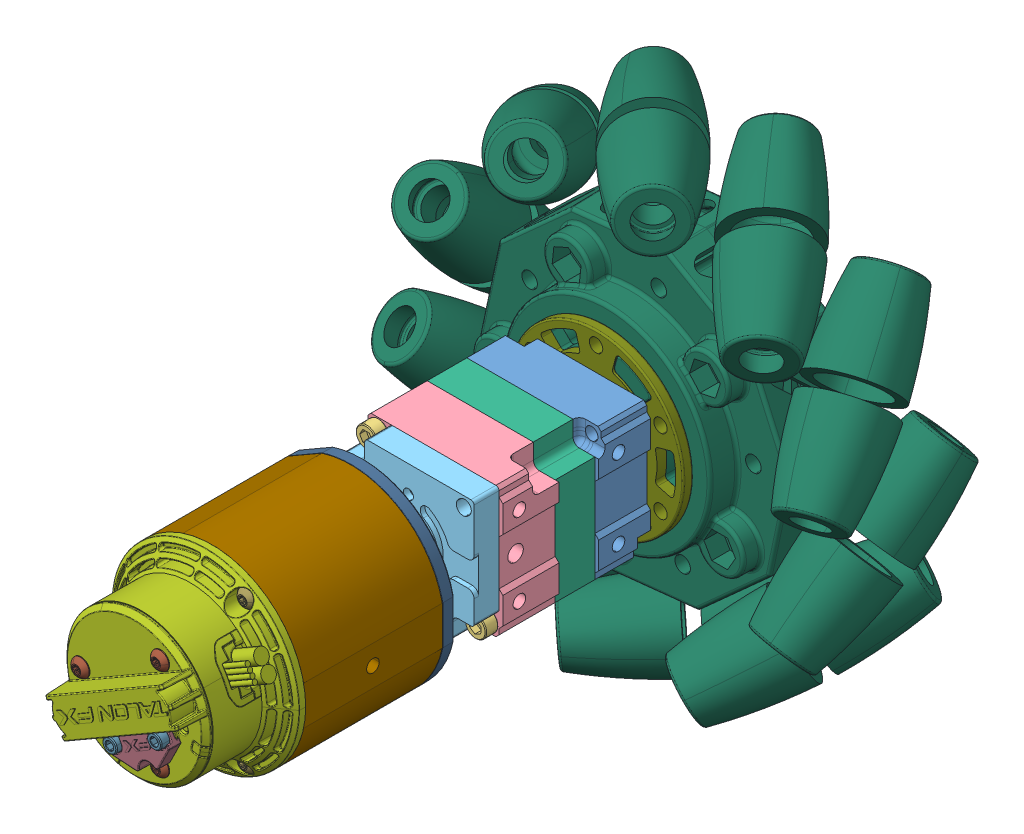
SolidWorks assembly RightMotorStack, configuration Default. Lengths in mm.
Overall size (178.38 178.3 209.52).
34 component instances, 27 part files, 5 mates.
Components (placement in the parent):
- MotorStack-1: MotorStack [Default] at (23.4756 40.0377 101.7362) size (81.62 81.39 192.35)
  - v2-VersaPlanetary-1stage-with-AM9015-20131031-1: v2-VersaPlanetary-1stage-with-AM9015-20131031 [Default] at (32.9453 91.261 18.2063) x (0 0 -1) z (0 1 0) size (95.9 44.45 42.1)
    - 217-2625-026 Rev1-1: 217-2625-026 Rev1 [Default] at (-6.5 22.225 0) x (0 -1 0) z (-1 0 0) size (44.45 42 18.13)
    - 217-2742-001 Rev4-1: 217-2742-001 Rev4 [Default] at (0.2002 22.225 0) x (1 0 0) z (0 -0.092627 0.995701) size (7 28 28)
    - 217-2742-001 Rev4-2: 217-2742-001 Rev4 [Default] at (8.2002 22.225 0) size (7 28 28)
    - 217-2625-017 Rev1_9714K61-1: 217-2625-017 Rev1_9714K61 [Default] at (7.42 22.3002 -0.342) x (0 0.56703 0.823697) z (0 -0.823697 0.56703) size (28.51 4.98 30.18)
    - 217-2625-003 Rev1-1: 217-2625-003 Rev1 [Default] at (7.4478 22.225 0) x (0 -1 0) z (1 0 0) size (17 17 64.12)
    - 217-2625-018 Rev1_98541A410-1: 217-2625-018 Rev1_98541A410 [Default] at (-0.7046 22.225 0) x (1 0 0) z (0 -0.017452 0.999848) size (1 19.6 17.4)
    - 832-1750-Ring-Gear-Screw_SSA0832-0500ZC-1: 832-1750-Ring-Gear-Screw_SSA0832-0500ZC [Default] at (-30.7 4.725 -17.5) x (0 0.997447 0.071411) z (0 -0.071411 0.997447) size (6.73 48.51 6.73)
    - 832-1750-Ring-Gear-Screw_SSA0832-0500ZC-2: 832-1750-Ring-Gear-Screw_SSA0832-0500ZC [Default] at (-30.7 39.725 17.5) x (0 0.005929 0.999982) z (0 -0.999982 0.005929) size (6.73 48.51 6.73)
    - 217-2625-025 Rev1-1: 217-2625-025 Rev1 [Default] at (-23.2 22.225 0) x (0 -1 0) z (-1 0 0) size (44.45 42 18)
    - 217-2822-004 Rev4-1: 217-2822-004 Rev4 [Default] at (-37.7 22.225 0) x (0 -1 0) z (-1 0 0) size (42 42 9.8)
    - 217-2820 Rev1_Public-1: 217-2820 Rev1_Public [Default] at (-4.6546 22.225 0) x (0 -0.456494 0.889726) z (-1 0 0)
      - 217-2625-100-1: 217-2625-100 [Default] at origin
    - 217-2816-001 Rev1-1: 217-2816-001 Rev1 [Default] at (-6.35 22.225 0) x (0 -1 0) z (1 0 0) size (42 42 14.5)
    - 217-4649-001 Rev1-1: 217-4649-001 Rev1 [Default] at (-20.046 22.225 0) x (0 -1 0) z (1 0 0) size (18 18 13)
    - 217-4649-007 Rev1_94105A824-1: 217-4649-007 Rev1_94105A824 [Default] at (-25.521 22.225 -6.7835) x (-0.996104 -0.088191 0) z (0 0 -1) size (4.83 4.83 4.9)
    - 217-2625-014 Rev2-1: 217-2625-014 Rev2 [Default] at (-24.7818 22.225 0) x (0 0 1) z (0 -1 0) size (8.01 7.5 7.94)
  - Falcon_500_Powered_by_Talon_FX_217-6515-1: Falcon_500_Powered_by_Talon_FX_217-6515 [Default] at (9.4877 97.4968 108.3478) x (1 0 0) z (0 0 -1) size (81.62 81.39 116.76)
    - Copy of 217-6515-Back 20190920^Falcon_500_Powered_by_Talon_FX_217-6515-1: Copy of 217-6515-Back 20190920^Falcon_500_Powered_by_Talon_FX_217-6515 [Default] at (1.2326 6.2358 -14.9619) size (60.06 60.12 79.55) (virtual)
    - Copy of Copy of 217-6515-201 Rev6^Falcon_500_Powered_by_Talon_FX_217-6515-1: Copy of Copy of 217-6515-201 Rev6^Falcon_500_Powered_by_Talon_FX_217-6515 [Default] at (1.2326 6.2358 50.6381) x (0.809017 0.587785 0) z (0 0 1) size (9.31 9.33 42.21) (virtual)
    - Copy of 217-6515-002 Rev6^Falcon_500_Powered_by_Talon_FX_217-6515-1: Copy of 217-6515-002 Rev6^Falcon_500_Powered_by_Talon_FX_217-6515 [Default] at (1.2326 6.2358 10.7381) x (0 -1 0) z (0 0 1) size (60 59.34 44.4) (virtual)
    - Copy of 217-6515-001 Rev6^Falcon_500_Powered_by_Talon_FX_217-6515-1: Copy of 217-6515-001 Rev6^Falcon_500_Powered_by_Talon_FX_217-6515 [Default] at (1.2326 6.2358 30.9381) x (0.5 0.866025 0) z (0 0 1) size (59.34 59.99 10) (virtual)
    - Copy of M3 BHTS-SECURE, Grade 8 Steel Rev1_SBTM3-24MMZB-SECURE^Falcon_500_Powered_by_Talon_FX_217-6515-1: Copy of M3 BHTS-SECURE, Grade 8 Steel Rev1_SBTM3-24MMZB-SECURE^Falcon_500_Powered_by_Talon_FX_217-6515 [Default] at (9.7324 20.9581 -38.0119) x (-0.923728 -0.383049 0) z (0 0 -1) size (5.69 5.69 25.65) (virtual)
    - Copy (2) of M3 BHTS-SECURE, Grade 8 Steel Rev1_SBTM3-24MMZB-SECURE^Falcon_500_Powered_by_Talon_FX_217-6515-2: Copy (2) of M3 BHTS-SECURE, Grade 8 Steel Rev1_SBTM3-24MMZB-SECURE^Falcon_500_Powered_by_Talon_FX_217-6515 [Default] at (-15.7672 6.2357 -38.0119) x (0.793594 -0.608447 0) z (0 0 -1) size (5.69 5.69 25.65) (virtual)
    - Copy (3) of M3 BHTS-SECURE, Grade 8 Steel Rev1_SBTM3-24MMZB-SECURE^Falcon_500_Powered_by_Talon_FX_217-6515-3: Copy (3) of M3 BHTS-SECURE, Grade 8 Steel Rev1_SBTM3-24MMZB-SECURE^Falcon_500_Powered_by_Talon_FX_217-6515 [Default] at (9.7326 -8.4864 -38.0119) x (0.130134 0.991496 0) z (0 0 -1) size (5.69 5.69 25.65) (virtual)
    - Copy of M3 BHTS, Grade 8 Steel Rev1_SBTM3-50MMZB^Falcon_500_Powered_by_Talon_FX_217-6515-1: Copy of M3 BHTS, Grade 8 Steel Rev1_SBTM3-50MMZB^Falcon_500_Powered_by_Talon_FX_217-6515 [Default] at (14.3576 28.969 -14.8619) x (-0.923728 -0.383049 0) z (0 0 -1) size (5.7 5.7 51.65) (virtual)
    - Copy (2) of M3 BHTS, Grade 8 Steel Rev1_SBTM3-50MMZB^Falcon_500_Powered_by_Talon_FX_217-6515-2: Copy (2) of M3 BHTS, Grade 8 Steel Rev1_SBTM3-50MMZB^Falcon_500_Powered_by_Talon_FX_217-6515 [Default] at (-25.0174 6.2358 -14.8619) x (0.793594 -0.608447 0) z (0 0 -1) size (5.7 5.7 51.65) (virtual)
    - Copy (3) of M3 BHTS, Grade 8 Steel Rev1_SBTM3-50MMZB^Falcon_500_Powered_by_Talon_FX_217-6515-3: Copy (3) of M3 BHTS, Grade 8 Steel Rev1_SBTM3-50MMZB^Falcon_500_Powered_by_Talon_FX_217-6515 [Default] at (14.3576 -16.4974 -14.8619) x (0.130134 0.991496 0) z (0 0 -1) size (5.7 5.7 51.65) (virtual)
    - Copy of 217-6515-308 Rev5^Falcon_500_Powered_by_Talon_FX_217-6515-1: Copy of 217-6515-308 Rev5^Falcon_500_Powered_by_Talon_FX_217-6515 [Default] at (7.0724 16.3512 -38.3619) x (0.866013 -0.500022 0) z (0.500022 0.866013 0) size (21.32 4.25 9.95) (virtual)
    - Copy of #4-40 SHCS, Grade 8 Steel Rev2_SSA0440-0125ZB^Falcon_500_Powered_by_Talon_FX_217-6515-1: Copy of #4-40 SHCS, Grade 8 Steel Rev2_SSA0440-0125ZB^Falcon_500_Powered_by_Talon_FX_217-6515 [Default] at (-1.3722 18.2247 -35.6869) x (-0.90374 0.428082 0) z (0 0 -1) size (4.65 4.65 6.03) (virtual)
    - Copy (2) of #4-40 SHCS, Grade 8 Steel Rev2_SSA0440-0125ZB^Falcon_500_Powered_by_Talon_FX_217-6515-2: Copy (2) of #4-40 SHCS, Grade 8 Steel Rev2_SSA0440-0125ZB^Falcon_500_Powered_by_Talon_FX_217-6515 [Default] at (12.917 9.9744 -35.6869) x (-0.992189 0.124742 0) z (0 0 -1) size (4.65 4.65 6.03) (virtual)
- Vex 6in Right-2: Vex 6in Right [Default] at (34.1959 131.2988 73.79) x (0.978148 -0.207912 0) z (0 0 1) size (150.41 150.31 56.44)
- MechanumHub-1: MechanumHub [Default] at (34.1959 131.2988 85.855) x (0 0 1) z (-0.5 -0.866025 0) size (12.7 55.88 55.88)
Mates (geometry in assembly coordinates):
- Coincident6: coincident anti-aligned: plane of Vex 6in Right-2 through (34.1959 131.2988 95.38) normal (0 0 1); plane of MechanumHub-1 through (21.8161 138.4462 95.38) normal (0 0 -1)
- Distance2: distance = 4.7625 mm anti-aligned: plane of MechanumHub-1 through (6.8756 147.0722 98.555) normal (0 0 1); plane of MotorStack-1/v2-VersaPlanetary-1stage-with-AM9015-20131031-1/217-2625-026 Rev1-1 through (11.9709 153.5238 103.3175) normal (0 0 -1)
- Concentric3: concentric anti-aligned: circle of MotorStack-1/v2-VersaPlanetary-1stage-with-AM9015-20131031-1/217-2625-026 Rev1-1; cylinder of MechanumHub-1 through (34.1959 131.2988 98.555) axis (0 0 1) radius 14.2949
- Parallel1: parallel anti-aligned: plane of MotorStack-1/v2-VersaPlanetary-1stage-with-AM9015-20131031-1/217-2625-003 Rev1-1 through (27.8459 127.6326 62.7423) normal (-1 0 0); plane of MechanumHub-1 through (27.8332 134.9723 85.855) normal (1 0 0)
- Concentric6: concentric aligned: cylinder of Vex 6in Right-2 through (13.5737 143.205 92.205) axis (0 0 1) radius 2.1526; cylinder of MechanumHub-1 through (13.5737 143.205 12.7617) axis (0 0 1) radius 2.15
